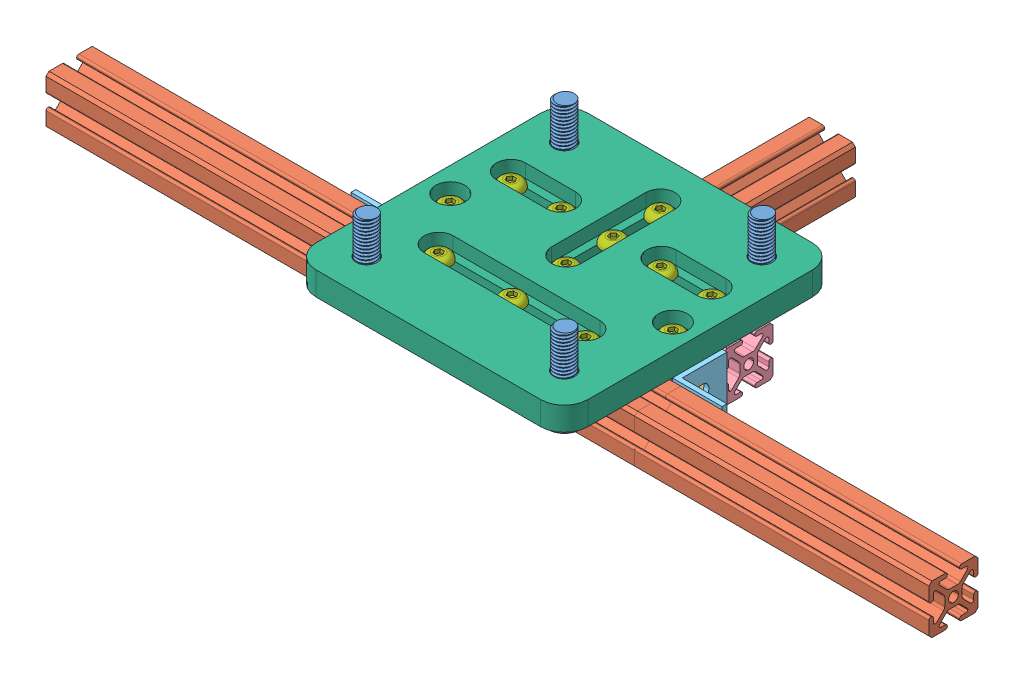
SolidWorks assembly Ouster_Assembly, configuration Default. Lengths in mm.
Overall size (357.53 44.91 162.95).
61 component instances, 13 part files, 63 mates.
Components (placement in the parent):
- 700-105333-04-OS1ExteriorSpec_BR.STEP-1: 700-105333-04-OS1ExteriorSpec_BR.STEP [Default] at origin size (200 96.59 200) (hidden)
  - 700-105333-OS1ExteriorSpec.STEP-1: 700-105333-OS1ExteriorSpec.STEP [Default] at origin size (87.01 58.35 85.37)
  - 700-105333-OS1ExteriorSpec_FOV.STEP-1: 700-105333-OS1ExteriorSpec_FOV.STEP [Default] at (0 2.002 0) size (200 72.84 200) (hidden)
  - 320-103537-TopCapAddOn_RadialFins_Ultra.STEP-1: 320-103537-TopCapAddOn_RadialFins_Ultra.STEP [Default] at origin size (80.38 21.38 80.38)
  - 320-102985-BasePlateOS01_HighFOV.SLDDRW_Option1.STEP-1: 320-102985-BasePlateOS01_HighFOV.SLDDRW_Option1.STEP [Default] at (0 -22.5 0) size (110 22.5 110)
  - 92855A307_TYPE 18-8 SS LOW PROFILE SOCKET CAP SCREW_92855A307.STEP-1: 92855A307_TYPE 18-8 SS LOW PROFILE SOCKET CAP SCREW_92855A307.STEP [Default] at (-21.2132 53.35 -21.2132) x (-0.408829 0 0.912611) z (0 -1 0) size (5.5 5.5 8.01)
  - 92855A307_TYPE 18-8 SS LOW PROFILE SOCKET CAP SCREW_92855A307.STEP-2: 92855A307_TYPE 18-8 SS LOW PROFILE SOCKET CAP SCREW_92855A307.STEP [Default] at (21.2132 53.35 -21.2132) x (-0.874587 0 -0.484869) z (0 -1 0) size (5.5 5.5 8.01)
  - 92855A307_TYPE 18-8 SS LOW PROFILE SOCKET CAP SCREW_92855A307.STEP-3: 92855A307_TYPE 18-8 SS LOW PROFILE SOCKET CAP SCREW_92855A307.STEP [Default] at (21.2132 53.35 21.2132) x (-0.944192 0 -0.329396) z (0 -1 0) size (5.5 5.5 8.01)
  - 92855A307_TYPE 18-8 SS LOW PROFILE SOCKET CAP SCREW_92855A307.STEP-4: 92855A307_TYPE 18-8 SS LOW PROFILE SOCKET CAP SCREW_92855A307.STEP [Default] at (-21.2132 53.35 21.2132) x (-0.999992 0 -0.003875) z (0 -1 0) size (5.5 5.5 8.01)
  - 92855A319_18-8 Stainless Steel Low-Profile Socket Head Screws_92855A319.STEP-1: 92855A319_18-8 Stainless Steel Low-Profile Socket Head Screws_92855A319.STEP [Default] at (-31.1769 2.5 18) x (-0.999881 0 0.015422) z (0 1 0) size (5.5 5.5 22.01)
  - 92855A319_18-8 Stainless Steel Low-Profile Socket Head Screws_92855A319.STEP-2: 92855A319_18-8 Stainless Steel Low-Profile Socket Head Screws_92855A319.STEP [Default] at (-18 2.5 -31.1769) x (-0.982062 0 -0.188556) z (0 1 0) size (5.5 5.5 22.01)
  - 92855A319_18-8 Stainless Steel Low-Profile Socket Head Screws_92855A319.STEP-3: 92855A319_18-8 Stainless Steel Low-Profile Socket Head Screws_92855A319.STEP [Default] at (18 2.5 -31.1769) x (0.692347 0 -0.721565) z (0 1 0) size (5.5 5.5 22.01)
  - 92855A319_18-8 Stainless Steel Low-Profile Socket Head Screws_92855A319.STEP-4: 92855A319_18-8 Stainless Steel Low-Profile Socket Head Screws_92855A319.STEP [Default] at (31.1769 2.5 18) x (0.996952 0 0.078023) z (0 1 0) size (5.5 5.5 22.01)
- A2_bolt.step-1: A2_bolt.step [Default] at (-39.9986 -32.025 -39.9986) size (13 33.05 13)
- A2_bolt.step-2: A2_bolt.step [Default] at (39.9986 -32.025 -39.9986) size (13 33.05 13)
- A2_bolt.step-3: A2_bolt.step [Default] at (39.9986 -32.025 39.9986) x (0.545679 0 -0.837994) z (0.837994 0 0.545679) size (13 33.05 13)
- A2_bolt.step-4: A2_bolt.step [Default] at (-39.9986 -32.025 39.9986) size (13 33.05 13)
- Alum_prof_resized-1: Alum_prof_resized [Default] at (0 -41.9564 -48.3654) size (19.86 19.86 119.18)
- Alum_prof_resized-2: Alum_prof_resized [Default] at (0 -41.9564 21.1544) x (0 1 0) z (1 0 0) size (19.86 19.86 119.18)
- Alum_prof_resized_shorter-1: Alum_prof_resized_shorter [Default] at (-45.0685 -41.9564 -48.3654) size (19.86 19.86 20.32)
- Alum_prof_resized_shorter-2: Alum_prof_resized_shorter [Default] at (45.0685 -41.9564 -48.3654) size (19.86 19.86 20.32)
- Alum_prof_resized-5: Alum_prof_resized [Default] at (-119.1768 -41.9564 21.1544) x (0 0 -1) z (1 0 0) size (19.86 19.86 119.18)
- Alum_prof_resized-6: Alum_prof_resized [Default] at (119.1768 -41.9564 21.1544) x (0 0 -1) z (1 0 0) size (19.86 19.86 119.18)
- Alum_prof_resized_short-1: Alum_prof_resized_short [Default] at (-69.5198 -41.9564 -19.0284) x (0 0 -1) z (1 0 0) size (19.86 19.86 45.72)
- Alum_prof_resized_short-2: Alum_prof_resized_short [Default] at (-3.937 -41.9564 -19.0284) x (0 0 -1) z (1 0 0) size (19.86 19.86 45.72)
- Corner-1: Corner [Default] at (-9.9314 -50.025 11.223) x (0 0 -1) z (0 -1 0) size (20.15 20.15 18)
- Corner-2: Corner [Default] at (9.9314 -50.025 11.223) x (1 0 0) z (0 -1 0) size (20.15 20.15 18)
- Corner-3: Corner [Default] at (54.9999 -50.025 11.223) x (1 0 0) z (0 -1 0) size (20.15 20.15 18)
- Corner-4: Corner [Default] at (-54.9999 -50.025 11.223) x (0 0 -1) z (0 -1 0) size (20.15 20.15 18)
- Corner-5: Corner [Default] at (9.9314 -50.025 -28.9598) x (1 0 0) z (0 -1 0) size (20.15 20.15 18)
- Corner-6: Corner [Default] at (-9.9314 -50.025 -28.9598) x (0 0 -1) z (0 -1 0) size (20.15 20.15 18)
- Corner-7: Corner [Default] at (35.1371 -50.025 -9.097) x (-1 0 0) z (0 -1 0) size (20.15 20.15 18)
- Corner-8: Corner [Default] at (-35.1371 -50.025 -9.097) x (0 0 1) z (0 -1 0) size (20.15 20.15 18)
- Assem1-1: Assem1 [Default] at origin size (110 15.51 110)
  - Old_Mount-1: Old_Mount [Default] at (0 -22.5 0) x (-1 0 0) z (0 1 0) size (110 110 9.53)
  - M5_Hex_Screw_Resized-1: M5_Hex_Screw_Resized [Default] at (-29.7053 -28.0118 21.1544) x (1 0 0) z (0 1 0) size (9.5 9.5 12.75)
  - M5_Hex_Screw_Resized-2: M5_Hex_Screw_Resized [Default] at (29.7053 -28.0118 21.1544) x (1 0 0) z (0 1 0) size (9.5 9.5 12.75)
  - M5_Hex_Screw_Resized-3: M5_Hex_Screw_Resized [Default] at (40.64 -28.0118 -19.0284) x (1 0 0) z (0 1 0) size (9.5 9.5 12.75)
  - M5_Hex_Screw_Resized-4: M5_Hex_Screw_Resized [Default] at (-45.0685 -28.0118 1.063) x (1 0 0) z (0 1 0) size (9.5 9.5 12.75)
  - M5_Hex_Screw_Resized-5: M5_Hex_Screw_Resized [Default] at (45.0685 -28.0118 1.063) x (1 0 0) z (0 1 0) size (9.5 9.5 12.75)
  - M5_Hex_Screw_Resized-6: M5_Hex_Screw_Resized [Default] at (20.32 -28.0118 -19.0284) x (1 0 0) z (0 1 0) size (9.5 9.5 12.75)
  - M5_Hex_Screw_Resized-7: M5_Hex_Screw_Resized [Default] at (-20.32 -28.0118 -19.0284) x (0.413777 0 0.910378) z (0 1 0) size (9.5 9.5 12.75)
  - M5_Hex_Screw_Resized-8: M5_Hex_Screw_Resized [Default] at (-40.64 -28.0118 -19.0284) x (1 0 0) z (0 1 0) size (9.5 9.5 12.75)
  - M5_Hex_Screw_Resized-9: M5_Hex_Screw_Resized [Default] at (0 -28.0118 21.1544) x (1 0 0) z (0 1 0) size (9.5 9.5 12.75)
  - M5_Hex_Screw_Resized-10: M5_Hex_Screw_Resized [Default] at (0 -28.0118 -0.8255) x (1 0 0) z (0 1 0) size (9.5 9.5 12.75)
  - M5_Hex_Screw_Resized-11: M5_Hex_Screw_Resized [Default] at (0 -28.0118 -38.9255) x (1 0 0) z (0 1 0) size (9.5 9.5 12.75)
  - M5_Hex_Screw_Resized-12: M5_Hex_Screw_Resized [Default] at (0 -28.0118 -19.8755) x (0.967917 0 0.25127) z (0 1 0) size (9.5 9.5 12.75)
- Assem1-2: Assem1 [Default] at (0 -83.9128 0) x (-1 0 0) z (0 0 1) size (110 15.51 110) (hidden)
  - Old_Mount-1: Old_Mount [Default] at (0 -22.5 0) x (-1 0 0) z (0 1 0) size (110 110 9.53)
  - M5_Hex_Screw_Resized-1: M5_Hex_Screw_Resized [Default] at (-29.7053 -28.0118 21.1544) x (1 0 0) z (0 1 0) size (9.5 9.5 12.75)
  - M5_Hex_Screw_Resized-2: M5_Hex_Screw_Resized [Default] at (29.7053 -28.0118 21.1544) x (1 0 0) z (0 1 0) size (9.5 9.5 12.75)
  - M5_Hex_Screw_Resized-3: M5_Hex_Screw_Resized [Default] at (40.64 -28.0118 -19.0284) x (1 0 0) z (0 1 0) size (9.5 9.5 12.75)
  - M5_Hex_Screw_Resized-4: M5_Hex_Screw_Resized [Default] at (-45.0685 -28.0118 1.063) x (1 0 0) z (0 1 0) size (9.5 9.5 12.75)
  - M5_Hex_Screw_Resized-5: M5_Hex_Screw_Resized [Default] at (45.0685 -28.0118 1.063) x (1 0 0) z (0 1 0) size (9.5 9.5 12.75)
  - M5_Hex_Screw_Resized-6: M5_Hex_Screw_Resized [Default] at (20.32 -28.0118 -19.0284) x (1 0 0) z (0 1 0) size (9.5 9.5 12.75)
  - M5_Hex_Screw_Resized-7: M5_Hex_Screw_Resized [Default] at (-20.32 -28.0118 -19.0284) x (0.413777 0 0.910378) z (0 1 0) size (9.5 9.5 12.75)
  - M5_Hex_Screw_Resized-8: M5_Hex_Screw_Resized [Default] at (-40.64 -28.0118 -19.0284) x (1 0 0) z (0 1 0) size (9.5 9.5 12.75)
  - M5_Hex_Screw_Resized-9: M5_Hex_Screw_Resized [Default] at (0 -28.0118 21.1544) x (1 0 0) z (0 1 0) size (9.5 9.5 12.75)
  - M5_Hex_Screw_Resized-10: M5_Hex_Screw_Resized [Default] at (0 -28.0118 -0.8255) x (1 0 0) z (0 1 0) size (9.5 9.5 12.75)
  - M5_Hex_Screw_Resized-11: M5_Hex_Screw_Resized [Default] at (0 -28.0118 -38.9255) x (1 0 0) z (0 1 0) size (9.5 9.5 12.75)
  - M5_Hex_Screw_Resized-12: M5_Hex_Screw_Resized [Default] at (0 -28.0118 -19.8755) x (0.967917 0 0.25127) z (0 1 0) size (9.5 9.5 12.75)
Mates (geometry in assembly coordinates):
- Coincident1: coordinate: point of 700-105333-04-OS1ExteriorSpec_BR.STEP-1
- Coincident16: coincident aligned: plane of Alum_prof_resized-1 through (0 -41.9564 -48.3654) normal (1 0 0)
- Coincident17: coincident aligned: plane of Alum_prof_resized-2 through (0 -41.9564 21.1544) normal (1 0 0)
- Coincident18: coincident anti-aligned: plane of Alum_prof_resized-1 through (0 -41.9564 11.223) normal (0 0 1); plane of Alum_prof_resized-2 through (59.5884 -41.9564 11.223) normal (0 0 -1)
- Coincident32: coincident aligned: plane of Alum_prof_resized-2 through (0 -41.9564 21.1544) normal (0 1 0); plane of Alum_prof_resized_shorter-1 through (-45.0685 -41.9564 -48.3654) normal (0 1 0)
- Coincident33: coincident anti-aligned: plane of Alum_prof_resized-2 through (59.5884 -41.9564 11.223) normal (0 0 -1); plane of Alum_prof_resized_shorter-1 through (-45.0685 -41.9564 11.223) normal (0 0 1)
- Coincident35: coincident anti-aligned: plane of Alum_prof_resized-2 through (59.5884 -41.9564 11.223) normal (0 0 -1); plane of Alum_prof_resized_shorter-2 through (45.0685 -41.9564 11.223) normal (0 0 1)
- Coincident37: coincident aligned: plane of Alum_prof_resized-2 through (0 -41.9564 21.1544) normal (0 1 0); plane of Alum_prof_resized_shorter-2 through (45.0685 -41.9564 -48.3654) normal (0 1 0)
- Coincident38: coincident aligned: plane of Alum_prof_resized-2 through (59.5884 -32.025 21.1544) normal (0 1 0); plane of Alum_prof_resized-6 through (178.7652 -32.025 21.1544) normal (0 1 0)
- Coincident39: coincident aligned: plane of Alum_prof_resized-2 through (59.5884 -41.9564 31.0858) normal (0 0 1); plane of Alum_prof_resized-6 through (178.7652 -41.9564 31.0858) normal (0 0 1)
- Coincident40: coincident aligned: plane of Alum_prof_resized-2 through (59.5884 -32.025 21.1544) normal (0 1 0); plane of Alum_prof_resized-5 through (-59.5884 -32.025 21.1544) normal (0 1 0)
- Coincident41: coincident aligned: plane of Alum_prof_resized-2 through (59.5884 -41.9564 31.0858) normal (0 0 1); plane of Alum_prof_resized-5 through (-59.5884 -41.9564 31.0858) normal (0 0 1)
- Coincident42: coincident anti-aligned: plane of Alum_prof_resized-2 through (59.5884 -41.9564 21.1544) normal (1 0 0); plane of Alum_prof_resized-6 through (59.5884 -41.9564 21.1544) normal (-1 0 0)
- Coincident43: coincident anti-aligned: plane of Alum_prof_resized-2 through (-59.5884 -41.9564 21.1544) normal (-1 0 0); plane of Alum_prof_resized-5 through (-59.5884 -41.9564 21.1544) normal (1 0 0)
- Coincident44: coincident aligned: plane of Alum_prof_resized-1 through (0 -32.025 11.223) normal (0 1 0); plane of Alum_prof_resized_short-1 through (-9.9314 -32.025 -19.0284) normal (0 1 0)
- Coincident45: coincident aligned: plane of Alum_prof_resized-1 through (0 -32.025 11.223) normal (0 1 0); plane of Alum_prof_resized_short-2 through (55.6514 -32.025 -19.0284) normal (0 1 0)
- Coincident46: coincident anti-aligned: plane of Alum_prof_resized-1 through (-9.9314 -41.9564 11.223) normal (-1 0 0); plane of Alum_prof_resized_short-1 through (-9.9314 -41.9564 -19.0284) normal (1 0 0)
- Coincident47: coincident anti-aligned: plane of Alum_prof_resized-1 through (9.9314 -41.9564 11.223) normal (1 0 0); plane of Alum_prof_resized_short-2 through (9.9314 -41.9564 -19.0284) normal (-1 0 0)
- Coincident48: coincident aligned: plane of Alum_prof_resized_short-1 through (-9.9314 -41.9564 -9.097) normal (0 0 1); plane of Alum_prof_resized_short-2 through (55.6514 -41.9564 -9.097) normal (0 0 1)
- Coincident49: coincident anti-aligned: plane of Alum_prof_resized_shorter-2 through (45.0685 -41.9564 -9.097) normal (0 0 -1); plane of Alum_prof_resized_short-2 through (55.6514 -41.9564 -9.097) normal (0 0 1)
- Coincident63: coincident anti-aligned: plane of Alum_prof_resized-5 through (-59.5884 -41.9564 11.223) normal (0 0 -1); plane of Corner-1 through (-9.9314 -32.025 11.223) normal (0 0 1)
- Coincident64: coincident anti-aligned: plane of Alum_prof_resized-1 through (-9.9314 -41.9564 11.223) normal (-1 0 0); plane of Corner-1 through (-9.9314 -32.025 11.223) normal (1 0 0)
- Coincident66: coincident aligned: plane of Alum_prof_resized-2 through (59.5884 -32.025 21.1544) normal (0 1 0); plane of Corner-1 through (-9.9314 -32.025 11.223) normal (0 1 0)
- Coincident67: coincident anti-aligned: plane of Alum_prof_resized_shorter-2 through (54.9999 -41.9564 11.223) normal (1 0 0); plane of Corner-3 through (54.9999 -32.025 11.223) normal (-1 0 0)
- Coincident68: coincident anti-aligned: plane of Alum_prof_resized-6 through (178.7652 -41.9564 11.223) normal (0 0 -1); plane of Corner-3 through (54.9999 -32.025 11.223) normal (0 0 1)
- Coincident69: coincident aligned: plane of Alum_prof_resized-6 through (178.7652 -32.025 21.1544) normal (0 1 0); plane of Corner-3 through (54.9999 -32.025 11.223) normal (0 1 0)
- Coincident70: coincident aligned: plane of Alum_prof_resized-5 through (-59.5884 -32.025 21.1544) normal (0 1 0); plane of Corner-4 through (-54.9999 -32.025 11.223) normal (0 1 0)
- Coincident71: coincident anti-aligned: plane of Alum_prof_resized-5 through (-59.5884 -41.9564 11.223) normal (0 0 -1); plane of Corner-4 through (-54.9999 -32.025 11.223) normal (0 0 1)
- Coincident72: coincident anti-aligned: plane of Alum_prof_resized_shorter-1 through (-54.9999 -41.9564 11.223) normal (-1 0 0); plane of Corner-4 through (-54.9999 -32.025 11.223) normal (1 0 0)
- Coincident73: coincident aligned: plane of Alum_prof_resized-1 through (0 -32.025 11.223) normal (0 1 0); plane of Corner-5 through (9.9314 -32.025 -28.9598) normal (0 1 0)
- Coincident74: coincident aligned: plane of Alum_prof_resized-1 through (0 -32.025 11.223) normal (0 1 0); plane of Corner-6 through (-9.9314 -32.025 -28.9598) normal (0 1 0)
- Coincident75: coincident anti-aligned: plane of Alum_prof_resized_short-2 through (55.6514 -41.9564 -28.9598) normal (0 0 -1); plane of Corner-5 through (9.9314 -32.025 -28.9598) normal (0 0 1)
- Coincident76: coincident anti-aligned: plane of Alum_prof_resized-1 through (9.9314 -41.9564 11.223) normal (1 0 0); plane of Corner-5 through (9.9314 -32.025 -28.9598) normal (-1 0 0)
- Coincident77: coincident anti-aligned: plane of Alum_prof_resized_short-1 through (-9.9314 -41.9564 -28.9598) normal (0 0 -1); plane of Corner-6 through (-9.9314 -32.025 -28.9598) normal (0 0 1)
- Coincident78: coincident anti-aligned: plane of Alum_prof_resized-1 through (-9.9314 -41.9564 11.223) normal (-1 0 0); plane of Corner-6 through (-9.9314 -32.025 -28.9598) normal (1 0 0)
- Coincident79: coincident aligned: plane of Alum_prof_resized_shorter-1 through (-45.0685 -32.025 11.223) normal (0 1 0); plane of Corner-8 through (-35.1371 -32.025 -9.097) normal (0 1 0)
- Coincident80: coincident anti-aligned: plane of Alum_prof_resized_shorter-1 through (-35.1371 -41.9564 11.223) normal (1 0 0); plane of Corner-8 through (-35.1371 -32.025 -9.097) normal (-1 0 0)
- Coincident81: coincident anti-aligned: plane of Alum_prof_resized_short-1 through (-9.9314 -41.9564 -9.097) normal (0 0 1); plane of Corner-8 through (-35.1371 -32.025 -9.097) normal (0 0 -1)
- Coincident82: coincident anti-aligned: plane of Alum_prof_resized-2 through (59.5884 -41.9564 11.223) normal (0 0 -1); plane of Corner-2 through (9.9314 -32.025 11.223) normal (0 0 1)
- Coincident83: coincident anti-aligned: plane of Alum_prof_resized-1 through (9.9314 -41.9564 11.223) normal (1 0 0); plane of Corner-2 through (9.9314 -32.025 11.223) normal (-1 0 0)
- Coincident84: coincident aligned: plane of Alum_prof_resized-2 through (59.5884 -32.025 21.1544) normal (0 1 0); plane of Corner-2 through (9.9314 -32.025 11.223) normal (0 1 0)
- Coincident85: coincident aligned: plane of Alum_prof_resized_shorter-2 through (45.0685 -32.025 11.223) normal (0 1 0); plane of Corner-7 through (35.1371 -32.025 -9.097) normal (0 1 0)
- Coincident86: coincident anti-aligned: plane of Alum_prof_resized_shorter-2 through (35.1371 -41.9564 11.223) normal (-1 0 0); plane of Corner-7 through (35.1371 -32.025 -9.097) normal (1 0 0)
- Coincident87: coincident anti-aligned: plane of Alum_prof_resized_short-2 through (55.6514 -41.9564 -9.097) normal (0 0 1); plane of Corner-7 through (35.1371 -32.025 -9.097) normal (0 0 -1)
- Coincident88: coincident anti-aligned: plane of Assem1-1/Old_Mount-1 through (0 -22.5 0) normal (-1 0 0)
- Coincident89: coincident anti-aligned: plane of 700-105333-04-OS1ExteriorSpec_BR.STEP-1/320-102985-BasePlateOS01_HighFOV.SLDDRW_Option1.STEP-1 through (-40 -22.5 -40) normal (0 -1 0); plane of Assem1-1/Old_Mount-1 through (0 -22.5 0) normal (0 1 0)
- Coincident90: coincident aligned: plane of Assem1-1/Old_Mount-1 through (0 -22.5 0) normal (0 0 1)
- Coincident91: coincident anti-aligned: plane of Assem1-1/Old_Mount-1 through (0 -32.025 0) normal (0 -1 0); plane of Alum_prof_resized-2 through (59.5884 -32.025 21.1544) normal (0 1 0)
- Coincident92: coincident anti-aligned: plane of Assem1-1/Old_Mount-1 through (0 -32.025 0) normal (0 -1 0); plane of Alum_prof_resized-1 through (0 -32.025 11.223) normal (0 1 0)
- Coincident93: coincident aligned: plane of Assem1-1/Old_Mount-1 through (0 -22.5 21.1544) normal (0 0 1); plane of Alum_prof_resized-2 through (0 -41.9564 21.1544) normal (0 0 1)
- Concentric18: concentric aligned: circle of Assem1-1/Old_Mount-1; circle of A2_bolt.step-1
- Coincident94: coincident anti-aligned: plane of Assem1-1/Old_Mount-1 through (0 -32.025 0) normal (0 -1 0); plane of A2_bolt.step-1 through (-39.9986 -32.025 -39.9986) normal (0 1 0)
- Concentric19: concentric aligned: circle of Assem1-1/Old_Mount-1; circle of A2_bolt.step-4
- Coincident95: coincident anti-aligned: plane of Assem1-1/Old_Mount-1 through (0 -32.025 0) normal (0 -1 0); plane of A2_bolt.step-4 through (-39.9986 -32.025 39.9986) normal (0 1 0)
- Concentric20: concentric aligned: circle of Assem1-1/Old_Mount-1; circle of A2_bolt.step-3
- Concentric21: concentric aligned: circle of Assem1-1/Old_Mount-1; circle of A2_bolt.step-2
- Coincident96: coincident anti-aligned: plane of Assem1-1/Old_Mount-1 through (0 -32.025 0) normal (0 -1 0); plane of A2_bolt.step-3 through (39.9986 -32.025 39.9986) normal (0 1 0)
- Coincident97: coincident anti-aligned: plane of Assem1-1/Old_Mount-1 through (0 -32.025 0) normal (0 -1 0); plane of A2_bolt.step-2 through (39.9986 -32.025 -39.9986) normal (0 1 0)
- Coincident98: coincident aligned: plane of Assem1-1/Old_Mount-1 through (-54.9999 -32.025 -54.9999) normal (-1 0 0); plane of Alum_prof_resized_shorter-1 through (-54.9999 -41.9564 11.223) normal (-1 0 0)
- Coincident99: coincident aligned: plane of Assem1-1/Old_Mount-1 through (54.9999 -32.025 -54.9999) normal (1 0 0); plane of Alum_prof_resized_shorter-2 through (54.9999 -41.9564 11.223) normal (1 0 0)
- Coincident100: coincident anti-aligned: plane of Alum_prof_resized-2 through (59.5884 -51.8878 21.1544) normal (0 -1 0); plane of Assem1-2/Old_Mount-1 through (0 -51.8878 0) normal (0 1 0)
- Coincident101: coincident aligned: plane of Assem1-1/Old_Mount-1 through (54.9999 -32.025 -54.9999) normal (0 0 -1); plane of Assem1-2/Old_Mount-1 through (-54.9999 -51.8878 -54.9999) normal (0 0 -1)
- Coincident102: coincident aligned: plane of Assem1-1/Old_Mount-1 through (-54.9999 -32.025 -54.9999) normal (-1 0 0); plane of Assem1-2/Old_Mount-1 through (-54.9999 -51.8878 -54.9999) normal (-1 0 0)
